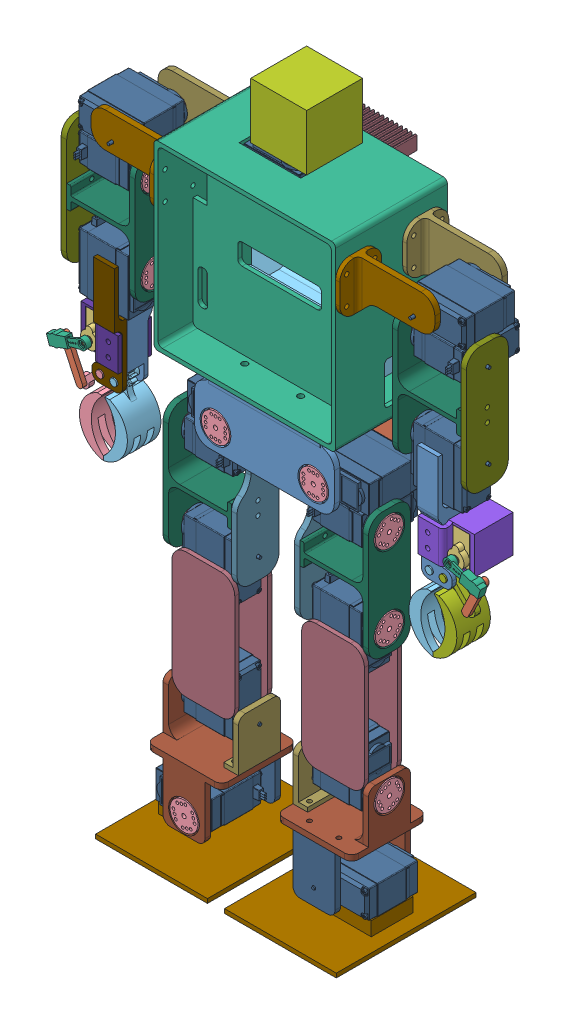
SolidWorks assembly Robot, configuration Default. Lengths in mm.
Overall size (371.9 484.07 152.92).
129 component instances, 32 part files, 19 mates.
Components (placement in the parent):
- Hip-1: Hip [Default] at (0 -77.1 -40) size (100 46.3 52) (flexible)
  - mh1-1: mh1 [Default] x (1 0 0) z (0 -1 0) size (100 52 44.45)
  - mh2-1: mh2 [Default] at (0 -26 -26) x (-1 0 0) z (0 0 1) size (100 40 15)
  - vb_1-1: vb_1 [Default] at (0 0.8 0) x (1 0 0) z (0 -1 0) size (50 50 2.3)
  - ktS-3: ktS [Default] at (-35 -29 26) x (1 0 0) z (0 0 -1) size (20 20 5.2)
  - ktS-4: ktS [Default] at (35 -29 26) x (1 0 0) z (0 0 -1) size (20 20 5.2)
- Body-1: Body [Default] at origin size (246 190.12 115.8) (flexible)
  - dp-1: dp [Default] at (-0.587 -1.3092 -49) x (-1 0 0) z (0 -1 0) size (87 49 112)
  - ktS-1: ktS [Default] at (1.0281 75.816 -38.25) x (0 0 -1) z (0 -1 0) size (20 20 5.2)
  - trb-1: trb [Default] x (1 0 0) z (0 0 -1) size (130 132.5 80)
  - uad-1: uad [Default] at (1.0281 93.816 -23.25) x (-1 0 0) z (0 0 -1) size (40 40 40)
  - vb_1-1: vb_1 [Default] at (0 -68.3 -40) x (-1 0 0) z (0 1 0) size (50 50 2.3)
  - vb_2-1: vb_2 [Default] at (0 -76.3 -40) x (0.999999 0 -0.001006) z (0 1 0) size (34.5 34.5 8)
  - vt-1: vt [Default] at (-65 35 -15) x (0 0 1) z (-1 0 0) size (30 35 58)
  - Servo_MG996-2: Servo_MG996 [Default] at (15.449 3.9516 -28.8898) x (-1 0 0) z (0 -1 0) size (48.16 20.5 52.7)
    - MG996R-1: MG996R [По умолчанию] at (25.0987 9.3602 39.3787) size (48.16 20.5 48.7)
    - MG996R Shaft-1: MG996R Shaft [Default] at (14.8987 9.3602 71.5787) x (1 0 0) z (0 -1 0) size (6 9 6)
  - Servo_MG996-4: Servo_MG996 [Default] at (15.9267 -2.7627 -47.6102) x (-1 0 0) z (0 1 0) size (48.16 20.5 52.7)
    - MG996R-1: MG996R [По умолчанию] at (25.0987 9.3602 39.3787) size (48.16 20.5 48.7)
    - MG996R Shaft-1: MG996R Shaft [Default] at (14.8987 9.3602 71.5787) x (1 0 0) z (0 -1 0) size (6 9 6)
  - vs-3: vs [Default] at (-65 35 -63) x (0 0 1) z (-1 0 0) size (30 35 58)
  - ktS-4: ktS [Default] at (-108 35 -65) size (20 20 5.2)
  - vt-3: vt [Default] at (65 35 -15) x (0 0 -1) z (1 0 0) size (30 35 58)
  - ktS-7: ktS [Default] at (108 35 -65) x (-1 0 0) z (0 0 1) size (20 20 5.2)
  - vs-6: vs [Default] at (65 35 -63) x (0 0 1) z (1 0 0) size (30 35 58)
  - poa-1: poa [Default] at (-0.5952 30.4748 -73.6) x (1 0 0) z (0 -1 0) size (79 49.8 120)
    - dcdc-1: dcdc [Default] at (29.3828 -3.2 19.6358) x (-1 0 0) z (0 0 1) size (60 29.45 53)
    - kp3-1: kp3 [Default] at origin size (79 23.8 60)
    - kp3-2: kp3 [Default] at (0 0 60) size (79 23.8 60)
- Left_Arm-1: Left_Arm [Default] at (-141 -15.5 -28.6) size (98.41 222.94 130.74) (flexible)
  - ktc_1-1: ktc_1 [Default] at (49 0 0) x (-1 0 0) z (0 -1 0) size (49 30 90)
  - ktc_2-1: ktc_2 [Default] x (-1 0 0) z (0 -1 0) size (4 30 90)
  - ktS-1: ktS [Default] at (49 30 0) x (0 1 0) z (-1 0 0) size (20 20 5.2)
  - Servo_MG996-1: Servo_MG996 [Default] at (-29.5787 -15.1013 9.3602) x (0 -1 0) z (1 0 0) size (48.16 20.5 52.7)
    - MG996R-1: MG996R [По умолчанию] at (25.0987 9.3602 39.3787) size (48.16 20.5 48.7)
    - MG996R Shaft-1: MG996R Shaft [Default] at (14.8987 9.3602 71.5787) x (1 0 0) z (0 -1 0) size (6 9 6)
  - ktS-2: ktS [Default] at (49 -30 0) x (0 1 0) z (-1 0 0) size (20 20 5.2)
  - Servo_MG996-2: Servo_MG996 [Default] at (47.8987 41.1398 42.1787) x (-1 0 0) z (0 0 -1) size (48.16 20.5 52.7)
    - MG996R-1: MG996R [По умолчанию] at (25.0987 9.3602 39.3787) size (48.16 20.5 48.7)
    - MG996R Shaft-1: MG996R Shaft [Default] at (14.8987 9.3602 71.5787) x (1 0 0) z (0 -1 0) size (6 9 6)
  - Servo_MG996-3: Servo_MG996 [Default] at (-29.5787 20.6398 14.8987) x (0 0 -1) z (1 0 0) size (48.16 20.5 52.7)
    - MG996R-1: MG996R [По умолчанию] at (25.0987 9.3602 39.3787) size (48.16 20.5 48.7)
    - MG996R Shaft-1: MG996R Shaft [Default] at (14.8987 9.3602 71.5787) x (1 0 0) z (0 -1 0) size (6 9 6)
  - Left_Hand-1: Left_Hand [Default] at (-9.6576 -119.8693 99.4752) x (0.26291 -0.876594 0.403065) z (0.964692 0.23201 -0.124664) size (127.58 78.42 65.96)
    - hdsvt-1: hdsvt [Default] at (-68.7677 84.8836 44.507) x (-0.26291 0.015765 -0.964692) z (0.876594 0.421608 -0.23201) size (33.5 34.6 26.6)
    - Ln-1: Ln [Default] at (-41.349 79.7943 49.8466) x (0.403065 -0.906641 -0.124664) z (0.26291 -0.015765 0.964692) size (9 82 22)
    - Lnp-1: Lnp [Default] at (-47.4784 93.574 51.7423) x (0.403065 -0.906641 -0.124664) z (0.26291 -0.015765 0.964692) size (18.2 82 22)
    - Lnt_-1: Lnt_ [Default] at (-47.8147 81.3076 19.5405) x (0.403065 -0.906641 -0.124664) z (0.906057 0.376153 0.193828) size (12 5 32)
    - Servo 9g-1: Servo 9g [Varsayılan] at (-74.611 92.0607 39.9971) x (-0.26291 0.015765 -0.964692) z (-0.876594 -0.421608 0.23201) size (12 30 24.1)
    - btc-1: btc [Default] at (-45.671 83.7599 40.7233) x (-0.403065 0.906641 0.124664) z (-0.253573 0.020247 -0.967104) size (24 55.74 25.45)
    - btt-1: btt [Default] at (-44.6542 87.2288 50.8689) x (0.403065 -0.906641 -0.124664) z (-0.873831 -0.421749 0.241966) size (24 18.18 56)
    - knsv_f-1: knsv_f [Default] at (-46.8154 63.2534 24.0615) x (0.036738 0.152139 -0.987676) z (-0.403065 0.906641 0.124664) size (27.71 8 6)
- Right_Arm-1: Right_Arm [Default] at (141 -15.5 -28.6) size (146.49 232.52 104.8) (flexible)
  - ktc_1-1: ktc_1 [Default] at (-49 0 0) x (1 0 0) z (0 -1 0) size (49 30 90)
  - ktc_2-1: ktc_2 [Default] x (1 0 0) z (0 -1 0) size (4 30 90)
  - ktS-1: ktS [Default] at (-49 30 0) x (0 1 0) z (1 0 0) size (20 20 5.2)
  - Servo_MG996-1: Servo_MG996 [Default] at (29.5787 -15.1013 -9.3602) x (0 -1 0) z (-1 0 0) size (48.16 20.5 52.7)
    - MG996R-1: MG996R [По умолчанию] at (25.0987 9.3602 39.3787) size (48.16 20.5 48.7)
    - MG996R Shaft-1: MG996R Shaft [Default] at (14.8987 9.3602 71.5787) x (1 0 0) z (0 -1 0) size (6 9 6)
  - MG996R-1: MG996R [По умолчанию] at (-9.8 30 -10.2) x (0 0 -1) z (-1 0 0) size (48.16 20.5 48.7)
  - MG996R Shaft-1: MG996R Shaft [Default] at (-42 30 0) x (0 0.937982 -0.346683) z (0 0.346683 0.937982) size (6 9 6)
  - MG996R-2: MG996R [По умолчанию] at (-22.8 50.5 2.8) x (1 0 0) z (0 0 -1) size (48.16 20.5 48.7)
  - MG996R Shaft-2: MG996R Shaft [Default] at (-33 50.5 -29.4) x (0.555138 0.831758 0) z (-0.831758 0.555138 0) size (6 9 6)
  - ktS-2: ktS [Default] at (-49 -30 0) x (0 1 0) z (1 0 0) size (20 20 5.2)
  - Right_Hand-1: Right_Hand [Default] at (97.3865 -82.637 -6.907) x (0.378084 -0.02914 -0.925313) z (-0.705847 0.637663 -0.308491) size (47.08 119.15 113.32)
    - btp-1: btp [Default] at (-48.4708 84.3864 63.4852) x (-0.925313 -0.220522 -0.308491) z (0.378372 -0.590807 -0.712588) size (24 55.74 25.27)
    - knsv_f-1: knsv_f [Default] at (-63.7619 51.2144 53.943) x (0.370894 -0.35693 -0.857344) z (0.925313 0.220522 0.308491) size (27.71 8 6)
    - Ln-1: Ln [Default] at (-48.5503 91.2587 71.7777) x (0.925313 0.220522 0.308491) z (-0.378084 0.599027 0.705847) size (9 82 22)
    - Lnp-1: Lnp [Default] at (-62.6151 87.9068 67.0886) x (0.925313 0.220522 0.308491) z (-0.378084 0.599027 0.705847) size (18.2 82 22)
    - Lnt_-1: Lnt_ [Default] at (-50.6565 70.957 43.9838) x (0.925313 0.220522 0.308491) z (0.137951 -0.953535 0.267844) size (12 5 32)
    - Servo 9g-1: Servo 9g [Varsayılan] at (-32.1005 66.5564 75.4283) x (-0.378084 0.599027 0.705847) z (-0.02914 -0.769764 0.637663) size (12 30 24.1)
    - btt-1: btt [Default] at (-55.9529 89.4945 69.3097) x (0.925313 0.220522 0.308491) z (-0.033045 -0.763534 0.644922) size (24 18.18 56)
    - hdsvp-1: hdsvp [Default] at (-42.041 68.5357 76.9244) x (0.378084 -0.599027 -0.705847) z (-0.02914 -0.769764 0.637663) size (33.5 34.6 26.6)
- Left_Leg-1: Left_Leg [Default] at (-46.4 -241.3 -19.75) size (80 274.4 100) (flexible)
  - bc-1: bc [Default] at (-0.8 -128.95 -10.75) x (0 0 -1) z (0 1 0) size (100 80 13)
  - ktS-1: ktS [Default] at (-27.1 114.7 -10.25) x (0 0.593175 0.805073) z (1 0 0) size (20 20 5.2)
  - mcc_1-1: mcc_1 [Default] at (-0.1 -77.2 -32) x (1 0 0) z (0 0 -1) size (30 40 10.5)
  - mcc_2-1: mcc_2 [Default] at (-0.1 -73.2 -10.25) x (0 -1 0) z (1 0 0) size (80 54 54)
  - mcc_3-1: mcc_3 [Default] at (21.65 -73.2 -10.25) x (0 1 0) z (0 0 1) size (36 10.5 30)
  - od-1: od [Default] at (0 0 -23.5) x (0 1 0) z (0 0 1) size (90 45 3)
  - Servo_MG996-1: Servo_MG996 [Default] at (14.7987 -96.3398 -61.8287) x (-1 0 0) z (0 0 1) size (48.16 20.5 52.7)
    - MG996R-1: MG996R [По умолчанию] at (25.0987 9.3602 39.3787) size (48.16 20.5 48.7)
    - MG996R Shaft-1: MG996R Shaft [Default] at (14.8987 9.3602 71.5787) x (1 0 0) z (0 -1 0) size (6 9 6)
  - ktc_1-1: ktc_1 [Default] at (-27.1 84.7 -10.25) x (1 0 0) z (0 1 0) size (49 30 90)
  - ktc_3-1: ktc_3 [Default] at (21.9 84.7 -10.25) x (1 0 0) z (0 1 0) size (4 30 90)
  - Servo_MG996-2: Servo_MG996 [Default] at (51.4787 69.5987 -19.6102) x (0 -1 0) z (-1 0 0) size (48.16 20.5 52.7)
    - MG996R-1: MG996R [По умолчанию] at (25.0987 9.3602 39.3787) size (48.16 20.5 48.7)
    - MG996R Shaft-1: MG996R Shaft [Default] at (14.8987 9.3602 71.5787) x (1 0 0) z (0 -1 0) size (6 9 6)
  - Servo_MG996-3: Servo_MG996 [Default] at (51.4787 -63.5987 -0.8898) x (0 1 0) z (-1 0 0) size (48.16 20.5 52.7)
    - MG996R-1: MG996R [По умолчанию] at (25.0987 9.3602 39.3787) size (48.16 20.5 48.7)
    - MG996R Shaft-1: MG996R Shaft [Default] at (14.8987 9.3602 71.5787) x (1 0 0) z (0 -1 0) size (6 9 6)
  - Servo_MG996-4: Servo_MG996 [Default] at (26.2987 144.5602 -72.8287) x (-1 0 0) z (0 0 1) size (48.16 20.5 52.7)
    - MG996R-1: MG996R [По умолчанию] at (25.0987 9.3602 39.3787) size (48.16 20.5 48.7)
    - MG996R Shaft-1: MG996R Shaft [Default] at (14.8987 9.3602 71.5787) x (1 0 0) z (0 -1 0) size (6 9 6)
  - ktS-2: ktS [Default] at (-0.1 -105.7 16.75) x (-0.959372 -0.282143 0) z (0 0 -1) size (20 20 5.2)
  - ktS-3: ktS [Default] at (-27.1 -48.7 -10.25) x (0 -0.912635 -0.408775) z (1 0 0) size (20 20 5.2)
  - ktS-4: ktS [Default] at (-27.1 54.7 -10.25) x (0 0.593175 0.805073) z (1 0 0) size (20 20 5.2)
  - od-2: od [Default] x (0 1 0) z (0 0 1) size (90 45 3)
  - Servo_MG996-5: Servo_MG996 [Default] at (51.4787 124.0602 4.6487) x (0 0 -1) z (-1 0 0) size (48.16 20.5 52.7)
    - MG996R-1: MG996R [По умолчанию] at (25.0987 9.3602 39.3787) size (48.16 20.5 48.7)
    - MG996R Shaft-1: MG996R Shaft [Default] at (14.8987 9.3602 71.5787) x (1 0 0) z (0 -1 0) size (6 9 6)
- Right_Leg-1: Right_Leg [Default] at (44.3 -241.3 -21.85) size (80 274.4 100) (flexible)
  - bc-1: bc [Default] at (0.8 -128.95 -8.55) x (0 0 1) z (0 1 0) size (100 80 13)
  - ktc_1-1: ktc_1 [Default] at (27.1 84.7 -10.25) x (-1 0 0) z (0 -1 0) size (49 30 90)
  - ktc_3-1: ktc_3 [Default] at (-25.9 84.7 -10.25) x (1 0 0) z (0 1 0) size (4 30 90)
  - ktS-1: ktS [Default] at (27.1 -48.7 -10.25) x (0 -0.404386 0.914588) z (-1 0 0) size (20 20 5.2)
  - mcc_1-1: mcc_1 [Default] at (0.1 -77.2 11.5) x (-1 0 0) z (0 0 1) size (30 40 10.5)
  - mcc_2-1: mcc_2 [Default] at (0.1 -73.2 -10.25) x (0 -1 0) z (-1 0 0) size (80 54 54)
  - mcc_3-1: mcc_3 [Default] at (-21.65 -73.2 -10.25) x (0 1 0) z (0 0 -1) size (36 10.5 30)
  - od-1: od [Default] x (0 -1 0) z (0 0 1) size (90 45 3)
  - Servo_MG996-1: Servo_MG996 [Default] at (-14.7987 -96.3398 41.3287) x (1 0 0) z (0 0 -1) size (48.16 20.5 52.7)
    - MG996R-1: MG996R [По умолчанию] at (25.0987 9.3602 39.3787) size (48.16 20.5 48.7)
    - MG996R Shaft-1: MG996R Shaft [Default] at (14.8987 9.3602 71.5787) x (1 0 0) z (0 -1 0) size (6 9 6)
  - Servo_MG996-2: Servo_MG996 [Default] at (-51.4787 -63.5987 -19.6102) x (0 1 0) z (1 0 0) size (48.16 20.5 52.7)
    - MG996R-1: MG996R [По умолчанию] at (25.0987 9.3602 39.3787) size (48.16 20.5 48.7)
    - MG996R Shaft-1: MG996R Shaft [Default] at (14.8987 9.3602 71.5787) x (1 0 0) z (0 -1 0) size (6 9 6)
  - Servo_MG996-3: Servo_MG996 [Default] at (-51.4787 69.5987 -0.8898) x (0 -1 0) z (1 0 0) size (48.16 20.5 52.7)
    - MG996R-1: MG996R [По умолчанию] at (25.0987 9.3602 39.3787) size (48.16 20.5 48.7)
    - MG996R Shaft-1: MG996R Shaft [Default] at (14.8987 9.3602 71.5787) x (1 0 0) z (0 -1 0) size (6 9 6)
  - Servo_MG996-4: Servo_MG996 [Default] at (-51.4787 105.3398 4.6487) x (0 0 -1) z (1 0 0) size (48.16 20.5 52.7)
    - MG996R-1: MG996R [По умолчанию] at (25.0987 9.3602 39.3787) size (48.16 20.5 48.7)
    - MG996R Shaft-1: MG996R Shaft [Default] at (14.8987 9.3602 71.5787) x (1 0 0) z (0 -1 0) size (6 9 6)
  - Servo_MG996-5: Servo_MG996 [Default] at (-24.1987 125.8398 -70.7287) size (48.16 20.5 52.7)
    - MG996R-1: MG996R [По умолчанию] at (25.0987 9.3602 39.3787) size (48.16 20.5 48.7)
    - MG996R Shaft-1: MG996R Shaft [Default] at (14.8987 9.3602 71.5787) x (1 0 0) z (0 -1 0) size (6 9 6)
  - ktS-2: ktS [Default] at (0.1 -105.7 -37.25) x (-0.474705 0.880145 0) z (0 0 1) size (20 20 5.2)
  - ktS-3: ktS [Default] at (27.1 54.7 -10.25) x (0 0.832364 -0.554229) z (-1 0 0) size (20 20 5.2)
  - ktS-4: ktS [Default] at (27.1 114.7 -10.25) x (0 0.813915 -0.580984) z (-1 0 0) size (20 20 5.2)
  - od-2: od [Default] at (0 0 -23.5) x (0 -1 0) z (0 0 1) size (90 45 3)
Mates (geometry in assembly coordinates):
- Concentric1: concentric anti-aligned: cylinder of Hip-1/vb_1-1 through (0 -76.3 -40) axis (0 1 0) radius 17.5; cylinder of Body-1/vb_2-1 through (0 -68.3 -40) axis (0 -1 0) radius 17.25
- Coincident1: coincident anti-aligned: plane of Hip-1/vb_1-1 through (0 -76.3 -40) normal (0 1 0); plane of Body-1/vb_2-1 through (0 -76.3 -40) normal (0 -1 0)
- Parallel4: parallel aligned: plane of Body-1/trb-1 through (0 0 -25) normal (0 0 1)
- Parallel6: parallel anti-aligned: plane of Body-1/trb-1 through (-65 -65 -80) normal (0 -1 0)
- Parallel5: parallel anti-aligned: plane of Body-1/trb-1 through (-65 -65 -80) normal (-1 0 0)
- Coincident9: coordinate: unknown of Body-1
- LimitAngle_hip: limit planar angle = 3.141593 rad: plane of assembly through (75 0 0) normal (1 0 0); plane of assembly; plane of Hip-1/mh1-1 through (-40 -81.1 -14) normal (-1 0 0)
- Concentric2: concentric anti-aligned: cylinder of Body-1/ktS-4 through (-108 35 -65) axis (0 0 1) radius 1.5; cylinder of Left_Arm-1/Servo_MG996-2/MG996R Shaft-1 through (-108 35 -56) axis (0 0 -1) radius 1.25
- Coincident11: coincident anti-aligned: plane of Body-1/ktS-4 through (-108 35 -63) normal (0 0 1); plane of Left_Arm-1/Servo_MG996-2/MG996R Shaft-1 through (-108 35 -63) normal (0 0 -1)
- LimitAngle_HorShoulder_left: limit planar angle = 3.141593 rad: plane of assembly through (-75 0 0) normal (-1 0 0); plane of Left_Arm-1/Servo_MG996-2/MG996R-1 through (-138.7 45.25 -46.3) normal (-1 0 0)
- Coincident13: coincident anti-aligned: plane of Body-1/ktS-7 through (108 35 -63) normal (0 0 1); plane of Right_Arm-1/MG996R Shaft-2 through (108 35 -63) normal (0 0 -1)
- Concentric3: concentric anti-aligned: cylinder of Body-1/ktS-7 through (108 35 -65) axis (0 0 1) radius 1.5; cylinder of Right_Arm-1/MG996R Shaft-2 through (108 35 -56) axis (0 0 -1) radius 1.25
- LimitAngle_HorShoulder_right: limit planar angle = 3.141593 rad: plane of assembly through (75 0 0) normal (1 0 0); plane of assembly; plane of Right_Arm-1/MG996R-2 through (97.7 24.75 -46.3) normal (-1 0 0)
- Concentric4: concentric anti-aligned: cylinder of Hip-1/ktS-3 through (-35 -106.1 -14) axis (0 0 -1) radius 1.5; cylinder of Left_Leg-1/Servo_MG996-4/MG996R Shaft-1 through (-35 -106.1 -23) axis (0 0 1) radius 1.25
- Coincident14: coincident anti-aligned: plane of Hip-1/ktS-3 through (-35 -106.1 -16) normal (0 0 -1); plane of Left_Leg-1/Servo_MG996-4/MG996R Shaft-1 through (-35 -106.1 -16) normal (0 0 1)
- LimitAngle_HorHip_Left: limit planar angle = 3.141593 rad: plane of assembly through (-50 0 0) normal (-1 0 0); plane of assembly; plane of Left_Leg-1/Servo_MG996-4/MG996R-1 through (-24.7 -116.35 -32.7) normal (1 0 0)
- Coincident16: coincident anti-aligned: plane of Hip-1/ktS-4 through (35 -106.1 -16) normal (0 0 -1); plane of Right_Leg-1/Servo_MG996-5/MG996R Shaft-1 through (35 -106.1 -16) normal (0 0 1)
- Concentric5: concentric anti-aligned: cylinder of Hip-1/ktS-4 through (35 -106.1 -14) axis (0 0 -1) radius 1.5; cylinder of Right_Leg-1/Servo_MG996-5/MG996R Shaft-1 through (35 -106.1 -23) axis (0 0 1) radius 1.25
- LimitAngle_HorHip_Right: limit planar angle = 3.141593 rad: plane of assembly through (50 0 0) normal (1 0 0); plane of Right_Leg-1/Servo_MG996-5/MG996R-1 through (24.7 -95.85 -32.7) normal (-1 0 0)
